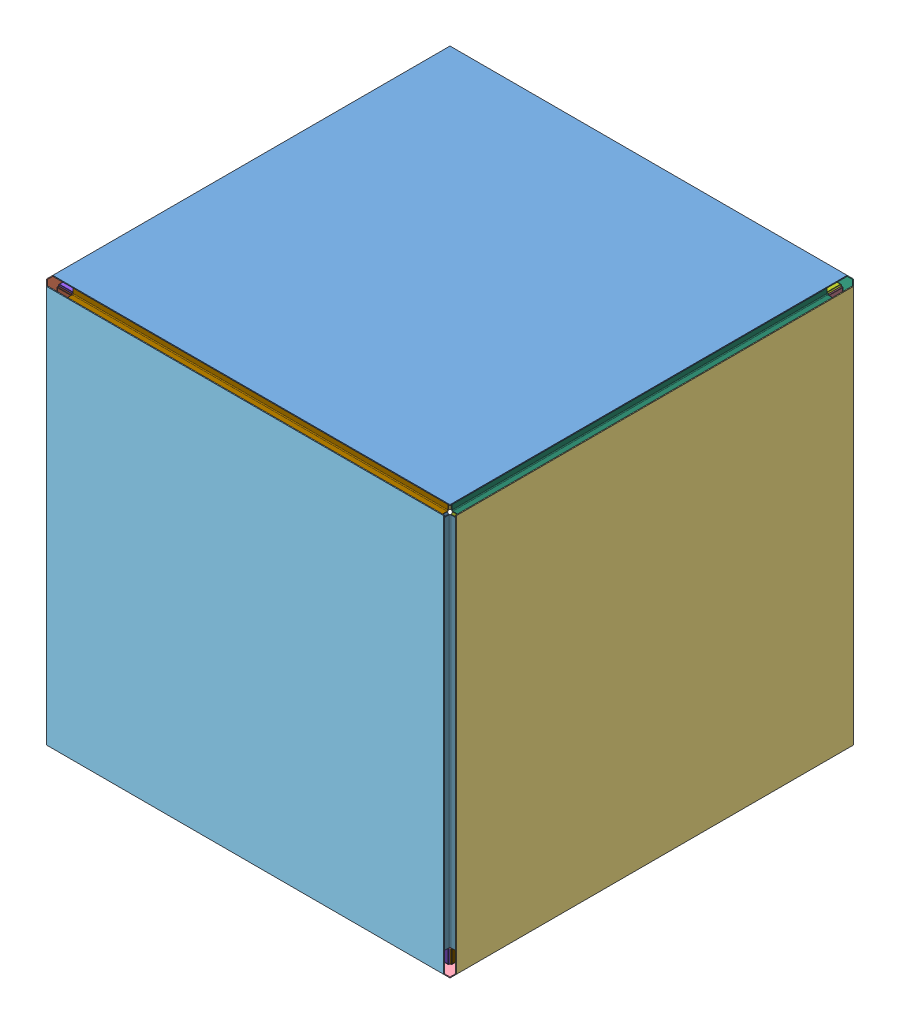
SolidWorks assembly cube_29, configuration cube29. Lengths in mm.
Overall size (714.38 714.38 714.38).
30 component instances, 30 part files, 93 mates.
Components (placement in the parent):
- pr^cube_29-28: pr^cube_29 [cube01] x (-1 0 0) z (0 0 1) size (692.15 1.59 692.15) (virtual)
- pg^cube_29-20: pg^cube_29 [cube01] x (0 -1 0) z (0 0 1) size (692.15 1.59 692.15) (virtual)
- po^cube_29-22: po^cube_29 [cube01] x (0 1 0) z (0 0 1) size (692.15 1.59 692.15) (virtual)
- py^cube_29-21: py^cube_29 [cube01] at origin size (692.15 1.59 692.15) (virtual)
- pc^cube_29-18: pc^cube_29 [cube01] x (-1 0 0) z (0 -1 0) size (692.15 1.59 692.15) (virtual)
- pb^cube_29-21: pb^cube_29 [cube01] x (-1 0 0) z (0 1 0) size (692.15 1.59 692.15) (virtual)
- br1^cube_29-49: br1^cube_29 [Default] at (0 330.2 -330.2) x (0 0 1) z (-1 0 0) size (50.8 50.8 653.29) (virtual)
- br2^cube_29-61: br2^cube_29 [Default] at (-330.2 330.2 0) size (50.8 50.8 653.29) (virtual)
- br3^cube_29-46: br3^cube_29 [Default] at (0 330.2 330.2) x (0 0 -1) z (1 0 0) size (50.8 50.8 653.29) (virtual)
- bg1^cube_29-47: bg1^cube_29 [Default] at (-330.2 -330.2 0) x (0 1 0) z (0 0 1) size (50.8 50.8 653.29) (virtual)
- bg2^cube_29-44: bg2^cube_29 [Default] at (-330.2 0 330.2) x (0 0 -1) z (0 1 0) size (50.8 50.8 653.29) (virtual)
- bg3^cube_29-40: bg3^cube_29 [Default] at (-330.2 0 -330.2) x (0 0 1) z (0 -1 0) size (50.8 50.8 653.29) (virtual)
- bo1^cube_29-42: bo1^cube_29 [Default] at (330.2 0 -330.2) x (0 0 1) z (0 1 0) size (50.8 50.8 653.29) (virtual)
- bo2^cube_29-46: bo2^cube_29 [Default] at (330.2 0 330.2) x (0 0 -1) z (0 -1 0) size (50.8 50.8 653.29) (virtual)
- bo3^cube_29-62: bo3^cube_29 [Default] at (330.2 330.2 0) x (0 -1 0) z (0 0 1) size (50.8 50.8 653.29) (virtual)
- by1^cube_29-41: by1^cube_29 [Default] at (0 -330.2 -330.2) x (0 0 1) z (1 0 0) size (50.8 50.8 653.29) (virtual)
- by2^cube_29-45: by2^cube_29 [Default] at (0 -330.2 330.2) x (0 0 -1) z (-1 0 0) size (50.8 50.8 653.29) (virtual)
- by3^cube_29-48: by3^cube_29 [Default] at (330.2 -330.2 0) x (-1 0 0) z (0 0 1) size (50.8 50.8 653.29) (virtual)
- dr1^cube_29-55: dr1^cube_29 [cube01] at (-354.9946 355.6 0) x (0 -1 0) z (0 0 1) size (26.01 26.01 711.21) (hidden, virtual)
- dr2^cube_29-37: dr2^cube_29 [cube01] at (0 355.6 354.9946) x (0 -1 0) z (1 0 0) size (26.01 26.01 711.21) (hidden, virtual)
- dr3^cube_29-33: dr3^cube_29 [cube01] at (0 355.6 -354.9946) x (0 -1 0) z (-1 0 0) size (26.01 26.01 711.21) (hidden, virtual)
- dg1^cube_29-38: dg1^cube_29 [cube01] at (-355.6 0 354.9946) x (1 0 0) z (0 1 0) size (26.01 26.01 711.21) (hidden, virtual)
- dg2^cube_29-41: dg2^cube_29 [cube01] at (-355.6 -354.9946 0) size (26.01 26.01 711.21) (hidden, virtual)
- dg3^cube_29-34: dg3^cube_29 [cube01] at (-355.6 0 -354.9946) x (1 0 0) z (0 -1 0) size (26.01 26.01 711.21) (hidden, virtual)
- do3^cube_29-47: do3^cube_29 [cube01] at (355.6 354.9946 0) x (-1 0 0) z (0 0 1) size (26.01 26.01 711.21) (hidden, virtual)
- do1^cube_29-36: do1^cube_29 [cube01] at (355.6 0 -354.9946) x (-1 0 0) z (0 1 0) size (26.01 26.01 711.21) (hidden, virtual)
- do2^cube_29-40: do2^cube_29 [cube01] at (355.6 0 354.9946) x (-1 0 0) z (0 -1 0) size (26.01 26.01 711.21) (hidden, virtual)
- dy1^cube_29-35: dy1^cube_29 [cube01] at (0 -355.6 -354.9946) x (0 1 0) z (1 0 0) size (26.01 26.01 711.21) (hidden, virtual)
- dy2^cube_29-39: dy2^cube_29 [cube01] at (0 -355.6 354.9946) x (0 1 0) z (-1 0 0) size (26.01 26.01 711.21) (hidden, virtual)
- dy3^cube_29-42: dy3^cube_29 [cube01] at (354.9946 -355.6 0) x (0 1 0) z (0 0 1) size (26.01 26.01 711.21) (hidden, virtual)
Mates (geometry in assembly coordinates):
- Coincident1: coincident anti-aligned: plane of pr^cube_29-28 through (346.075 355.6 -346.075) normal (0 -1 0); plane of br1^cube_29-49 through (-326.644 355.6 -330.2) normal (0 1 0)
- Coincident2: coincident anti-aligned: plane of pr^cube_29-28 through (346.075 355.6 -346.075) normal (0 -1 0); plane of br2^cube_29-61 through (-330.2 355.6 326.644) normal (0 1 0)
- Coincident3: coincident anti-aligned: plane of pr^cube_29-28 through (346.075 355.6 -346.075) normal (0 -1 0); plane of br3^cube_29-46 through (326.644 355.6 330.2) normal (0 1 0)
- Coincident4: coincident anti-aligned: plane of pr^cube_29-28 through (346.075 355.6 -346.075) normal (0 -1 0); plane of bo3^cube_29-62 through (330.2 355.6 326.644) normal (0 1 0)
- Coincident5: coincident anti-aligned: plane of pr^cube_29-28 through (346.075 355.6 -346.075) normal (0 -1 0); plane of dr3^cube_29-33 through (0 355.6 -710.5946) normal (0 1 0)
- Coincident6: coincident anti-aligned: plane of pr^cube_29-28 through (346.075 355.6 -346.075) normal (0 -1 0); plane of dr1^cube_29-55 through (-710.5946 355.6 0) normal (0 1 0)
- Coincident7: coincident anti-aligned: plane of pr^cube_29-28 through (346.075 355.6 -346.075) normal (0 -1 0); plane of do3^cube_29-47 through (-0.6054 355.6 0) normal (0 1 0)
- Coincident8: coincident anti-aligned: plane of pr^cube_29-28 through (346.075 355.6 -346.075) normal (0 -1 0); plane of dr2^cube_29-37 through (0 355.6 710.5946) normal (0 1 0)
- Coincident34: coincident anti-aligned: plane of pb^cube_29-21 through (346.075 -346.075 -355.6) normal (0 0 1); plane of by1^cube_29-41 through (326.644 -330.2 -355.6) normal (0 0 -1)
- Coincident35: coincident anti-aligned: plane of pb^cube_29-21 through (346.075 -346.075 -355.6) normal (0 0 1); plane of bo1^cube_29-42 through (330.2 326.644 -355.6) normal (0 0 -1)
- Coincident36: coincident anti-aligned: plane of pb^cube_29-21 through (346.075 -346.075 -355.6) normal (0 0 1); plane of br1^cube_29-49 through (-326.644 330.2 -355.6) normal (0 0 -1)
- Coincident37: coincident anti-aligned: plane of pb^cube_29-21 through (346.075 -346.075 -355.6) normal (0 0 1); plane of bg3^cube_29-40 through (-330.2 -326.644 -355.6) normal (0 0 -1)
- Coincident38: coincident anti-aligned: plane of pb^cube_29-21 through (346.075 -346.075 -355.6) normal (0 0 1); plane of dg3^cube_29-34 through (0.6054 0 -355.6) normal (0 0 -1)
- Coincident39: coincident anti-aligned: plane of pb^cube_29-21 through (346.075 -346.075 -355.6) normal (0 0 1); plane of dr3^cube_29-33 through (0 -0.6054 -355.6) normal (0 0 -1)
- Coincident40: coincident anti-aligned: plane of pb^cube_29-21 through (346.075 -346.075 -355.6) normal (0 0 1); plane of do1^cube_29-36 through (-0.6054 0 -355.6) normal (0 0 -1)
- Coincident41: coincident anti-aligned: plane of pb^cube_29-21 through (346.075 -346.075 -355.6) normal (0 0 1); plane of dy1^cube_29-35 through (0 0.6054 -355.6) normal (0 0 -1)
- Coincident42: coincident anti-aligned: plane of pc^cube_29-18 through (346.075 346.075 355.6) normal (0 0 -1); plane of bo2^cube_29-46 through (330.2 -326.644 355.6) normal (0 0 1)
- Coincident43: coincident anti-aligned: plane of pc^cube_29-18 through (346.075 346.075 355.6) normal (0 0 -1); plane of br3^cube_29-46 through (326.644 330.2 355.6) normal (0 0 1)
- Coincident44: coincident anti-aligned: plane of pc^cube_29-18 through (346.075 346.075 355.6) normal (0 0 -1); plane of bg2^cube_29-44 through (-330.2 326.644 355.6) normal (0 0 1)
- Coincident45: coincident anti-aligned: plane of pc^cube_29-18 through (346.075 346.075 355.6) normal (0 0 -1); plane of by2^cube_29-45 through (-326.644 -330.2 355.6) normal (0 0 1)
- Coincident46: coincident anti-aligned: plane of pc^cube_29-18 through (346.075 346.075 355.6) normal (0 0 -1); plane of do2^cube_29-40 through (-0.6054 0 355.6) normal (0 0 1)
- Coincident47: coincident anti-aligned: plane of pc^cube_29-18 through (346.075 346.075 355.6) normal (0 0 -1); plane of dy2^cube_29-39 through (0 0.6054 355.6) normal (0 0 1)
- Coincident48: coincident anti-aligned: plane of pc^cube_29-18 through (346.075 346.075 355.6) normal (0 0 -1); plane of dg1^cube_29-38 through (0.6054 0 355.6) normal (0 0 1)
- Coincident49: coincident anti-aligned: plane of pc^cube_29-18 through (346.075 346.075 355.6) normal (0 0 -1); plane of dr2^cube_29-37 through (0 -0.6054 355.6) normal (0 0 1)
- Coincident50: coincident anti-aligned: plane of pg^cube_29-20 through (-355.6 346.075 -346.075) normal (1 0 0); plane of bg3^cube_29-40 through (-355.6 -326.644 -330.2) normal (-1 0 0)
- Coincident51: coincident anti-aligned: plane of pg^cube_29-20 through (-355.6 346.075 -346.075) normal (1 0 0); plane of bg1^cube_29-47 through (-355.6 -330.2 326.644) normal (-1 0 0)
- Coincident52: coincident anti-aligned: plane of pg^cube_29-20 through (-355.6 346.075 -346.075) normal (1 0 0); plane of bg2^cube_29-44 through (-355.6 326.644 330.2) normal (-1 0 0)
- Coincident53: coincident anti-aligned: plane of pg^cube_29-20 through (-355.6 346.075 -346.075) normal (1 0 0); plane of dr1^cube_29-55 through (-355.6 -0.6054 0) normal (-1 0 0)
- Coincident54: coincident anti-aligned: plane of pg^cube_29-20 through (-355.6 346.075 -346.075) normal (1 0 0); plane of dg3^cube_29-34 through (-355.6 0 -710.5946) normal (-1 0 0)
- Coincident55: coincident anti-aligned: plane of pg^cube_29-20 through (-355.6 346.075 -346.075) normal (1 0 0); plane of dg2^cube_29-41 through (-355.6 -710.5946 0) normal (-1 0 0)
- Coincident56: coincident anti-aligned: plane of pg^cube_29-20 through (-355.6 346.075 -346.075) normal (1 0 0); plane of dg1^cube_29-38 through (-355.6 0 710.5946) normal (-1 0 0)
- Coincident99: coincident anti-aligned: plane of pg^cube_29-20 through (-355.6 346.075 -346.075) normal (1 0 0); plane of br2^cube_29-61 through (-355.6 330.2 326.644) normal (-1 0 0)
- Coincident57: coincident anti-aligned: plane of py^cube_29-21 through (-346.075 -355.6 -346.075) normal (0 1 0); plane of by3^cube_29-48 through (330.2 -355.6 326.644) normal (0 -1 0)
- Coincident58: coincident anti-aligned: plane of py^cube_29-21 through (-346.075 -355.6 -346.075) normal (0 1 0); plane of by2^cube_29-45 through (-326.644 -355.6 330.2) normal (0 -1 0)
- Coincident59: coincident anti-aligned: plane of py^cube_29-21 through (-346.075 -355.6 -346.075) normal (0 1 0); plane of bg1^cube_29-47 through (-330.2 -355.6 326.644) normal (0 -1 0)
- Coincident60: coincident anti-aligned: plane of py^cube_29-21 through (-346.075 -355.6 -346.075) normal (0 1 0); plane of by1^cube_29-41 through (326.644 -355.6 -330.2) normal (0 -1 0)
- Coincident61: coincident anti-aligned: plane of py^cube_29-21 through (-346.075 -355.6 -346.075) normal (0 1 0); plane of dy3^cube_29-42 through (710.5946 -355.6 0) normal (0 -1 0)
- Coincident62: coincident anti-aligned: plane of py^cube_29-21 through (-346.075 -355.6 -346.075) normal (0 1 0); plane of dy2^cube_29-39 through (0 -355.6 710.5946) normal (0 -1 0)
- Coincident63: coincident anti-aligned: plane of py^cube_29-21 through (-346.075 -355.6 -346.075) normal (0 1 0); plane of dg2^cube_29-41 through (0.6054 -355.6 0) normal (0 -1 0)
- Coincident64: coincident anti-aligned: plane of py^cube_29-21 through (-346.075 -355.6 -346.075) normal (0 1 0); plane of dy1^cube_29-35 through (0 -355.6 -710.5946) normal (0 -1 0)
- Coincident65: coincident anti-aligned: plane of po^cube_29-22 through (355.6 -346.075 -346.075) normal (-1 0 0); plane of bo1^cube_29-42 through (355.6 326.644 -330.2) normal (1 0 0)
- Coincident66: coincident anti-aligned: plane of po^cube_29-22 through (355.6 -346.075 -346.075) normal (-1 0 0); plane of by3^cube_29-48 through (355.6 -330.2 326.644) normal (1 0 0)
- Coincident67: coincident anti-aligned: plane of po^cube_29-22 through (355.6 -346.075 -346.075) normal (-1 0 0); plane of bo2^cube_29-46 through (355.6 -326.644 330.2) normal (1 0 0)
- Coincident68: coincident anti-aligned: plane of po^cube_29-22 through (355.6 -346.075 -346.075) normal (-1 0 0); plane of bo3^cube_29-62 through (355.6 330.2 326.644) normal (1 0 0)
- Coincident69: coincident anti-aligned: plane of po^cube_29-22 through (355.6 -346.075 -346.075) normal (-1 0 0); plane of do2^cube_29-40 through (355.6 0 710.5946) normal (1 0 0)
- Coincident70: coincident anti-aligned: plane of po^cube_29-22 through (355.6 -346.075 -346.075) normal (-1 0 0); plane of do3^cube_29-47 through (355.6 710.5946 0) normal (1 0 0)
- Coincident71: coincident anti-aligned: plane of po^cube_29-22 through (355.6 -346.075 -346.075) normal (-1 0 0); plane of do1^cube_29-36 through (355.6 0 -710.5946) normal (1 0 0)
- Coincident72: coincident anti-aligned: plane of po^cube_29-22 through (355.6 -346.075 -346.075) normal (-1 0 0); plane of dy3^cube_29-42 through (355.6 0.6054 0) normal (1 0 0)
- Coincident73: coincident aligned: plane of assembly through (0 0 0) normal (0 0 1); plane of dy3^cube_29-42 through (354.9946 -355.6 0) normal (0 0 1)
- Coincident74: coincident aligned: plane of assembly through (0 0 0) normal (0 0 1); plane of by3^cube_29-48 through (330.2 -330.2 0) normal (0 0 1)
- Coincident75: coincident aligned: plane of assembly through (0 0 0) normal (0 0 1); plane of bo3^cube_29-62 through (330.2 330.2 0) normal (0 0 1)
- Coincident76: coincident aligned: plane of assembly through (0 0 0) normal (0 0 1); plane of do3^cube_29-47 through (355.6 354.9946 0) normal (0 0 1)
- Coincident77: coincident aligned: plane of assembly through (0 0 0) normal (0 0 1); plane of dg2^cube_29-41 through (-355.6 -354.9946 0) normal (0 0 1)
- Coincident78: coincident aligned: plane of assembly through (0 0 0) normal (0 0 1); plane of bg1^cube_29-47 through (-330.2 -330.2 0) normal (0 0 1)
- Coincident79: coincident aligned: plane of assembly through (0 0 0) normal (0 0 1); plane of dr1^cube_29-55 through (-354.9946 355.6 0) normal (0 0 1)
- Coincident80: coincident aligned: plane of assembly through (0 0 0) normal (0 0 1); plane of br2^cube_29-61 through (-330.2 330.2 0) normal (0 0 1)
- Coincident81: coincident aligned: plane of assembly through (0 0 0) normal (0 1 0); plane of bo1^cube_29-42 through (330.2 0 -330.2) normal (0 1 0)
- Coincident82: coincident aligned: plane of assembly through (0 0 0) normal (0 1 0); plane of py^cube_29-21 through (0 0 0) normal (0 1 0)
- Coincident83: coincident aligned: plane of assembly through (0 0 0) normal (0 1 0); plane of do1^cube_29-36 through (355.6 0 -354.9946) normal (0 1 0)
- Coincident84: coincident anti-aligned: plane of assembly through (0 0 0) normal (0 1 0); plane of bg3^cube_29-40 through (-330.2 0 -330.2) normal (0 -1 0)
- Coincident85: coincident anti-aligned: plane of assembly through (0 0 0) normal (0 1 0); plane of dg3^cube_29-34 through (-355.6 0 -354.9946) normal (0 -1 0)
- Coincident86: coincident aligned: plane of assembly through (0 0 0) normal (0 1 0); plane of dg1^cube_29-38 through (-355.6 0 354.9946) normal (0 1 0)
- Coincident87: coincident aligned: plane of assembly through (0 0 0) normal (0 1 0); plane of bg2^cube_29-44 through (-330.2 0 330.2) normal (0 1 0)
- Coincident88: coincident anti-aligned: plane of assembly through (0 0 0) normal (0 1 0); plane of bo2^cube_29-46 through (330.2 0 330.2) normal (0 -1 0)
- Coincident89: coincident anti-aligned: plane of assembly through (0 0 0) normal (0 1 0); plane of do2^cube_29-40 through (355.6 0 354.9946) normal (0 -1 0)
- Coincident90: coincident anti-aligned: plane of assembly through (0 0 0) normal (1 0 0); plane of by2^cube_29-45 through (0 -330.2 330.2) normal (-1 0 0)
- Coincident91: coincident anti-aligned: plane of assembly through (0 0 0) normal (1 0 0); plane of dy2^cube_29-39 through (0 -355.6 354.9946) normal (-1 0 0)
- Coincident92: coincident aligned: plane of assembly through (0 0 0) normal (1 0 0); plane of pg^cube_29-20
- Coincident93: coincident aligned: plane of assembly through (0 0 0) normal (1 0 0); plane of dr2^cube_29-37 through (0 355.6 354.9946) normal (1 0 0)
- Coincident94: coincident aligned: plane of assembly through (0 0 0) normal (1 0 0); plane of br3^cube_29-46 through (0 330.2 330.2) normal (1 0 0)
- Coincident95: coincident anti-aligned: plane of assembly through (0 0 0) normal (1 0 0); plane of dr3^cube_29-33 through (0 355.6 -354.9946) normal (-1 0 0)
- Coincident96: coincident anti-aligned: plane of assembly through (0 0 0) normal (1 0 0); plane of br1^cube_29-49 through (0 330.2 -330.2) normal (-1 0 0)
- Coincident97: coincident aligned: plane of assembly through (0 0 0) normal (1 0 0); plane of by1^cube_29-41 through (0 -330.2 -330.2) normal (1 0 0)
- Coincident98: coincident aligned: plane of assembly through (0 0 0) normal (1 0 0); plane of dy1^cube_29-35 through (0 -355.6 -354.9946) normal (1 0 0)
- Coincident100: coincident anti-aligned: plane of pr^cube_29-28; plane of assembly through (0 0 0) normal (1 0 0)
- Coincident101: coincident aligned: plane of pr^cube_29-28 through (0 0 0) normal (0 0 1); plane of assembly through (0 0 0) normal (0 0 1)
- Coincident102: coincident anti-aligned: plane of pr^cube_29-28; plane of assembly through (0 0 0) normal (0 1 0)
- Coincident106: coincident anti-aligned: plane of pg^cube_29-20; plane of assembly through (0 0 0) normal (0 1 0)
- Coincident107: coincident aligned: plane of pg^cube_29-20; plane of assembly through (0 0 0) normal (1 0 0)
- Coincident108: coincident aligned: plane of pg^cube_29-20 through (0 0 0) normal (0 0 1); plane of assembly through (0 0 0) normal (0 0 1)
- Coincident109: coincident aligned: plane of py^cube_29-21 through (0 0 0) normal (0 0 1); plane of assembly through (0 0 0) normal (0 0 1)
- Coincident110: coincident aligned: plane of py^cube_29-21 through (0 0 0) normal (0 1 0); plane of assembly through (0 0 0) normal (0 1 0)
- Coincident111: coincident aligned: plane of py^cube_29-21 through (0 0 0) normal (1 0 0); plane of assembly through (0 0 0) normal (1 0 0)
- Coincident112: coincident aligned: plane of po^cube_29-22 through (0 0 0) normal (0 0 1); plane of assembly through (0 0 0) normal (0 0 1)
- Coincident113: coincident anti-aligned: plane of po^cube_29-22; plane of assembly through (0 0 0) normal (1 0 0)
- Coincident114: coincident aligned: plane of po^cube_29-22; plane of assembly through (0 0 0) normal (0 1 0)
- Coincident115: coincident anti-aligned: plane of pc^cube_29-18 through (0 0 0) normal (0 -1 0); plane of assembly through (0 0 0) normal (0 1 0)
- Coincident116: coincident anti-aligned: plane of pc^cube_29-18; plane of assembly through (0 0 0) normal (0 0 1)
- Coincident117: coincident anti-aligned: plane of pc^cube_29-18; plane of assembly through (0 0 0) normal (1 0 0)
- Coincident118: coincident aligned: plane of pb^cube_29-21 through (0 0 0) normal (0 1 0); plane of assembly through (0 0 0) normal (0 1 0)
- Coincident119: coincident aligned: plane of pb^cube_29-21; plane of assembly through (0 0 0) normal (0 0 1)
- Coincident120: coincident anti-aligned: line of pb^cube_29-21 through (0.8731 -0.8731 0) axis (0 0 -1); sketch_entity of pr^cube_29-28; plane of pb^cube_29-21 through (346.075 -346.075 -357.1875) normal (0 0 -1); plane of py^cube_29-21 through (-346.075 -357.1875 -346.075) normal (0 -1 0)
- cyan_cut: unknown: unknown of pc^cube_29-18; plane of pc^cube_29-18 through (346.075 346.075 357.1875) normal (0 0 1); plane of pg^cube_29-20 through (-357.1875 346.075 -346.075) normal (-1 0 0); plane of po^cube_29-22 through (357.1875 -346.075 -346.075) normal (1 0 0)
